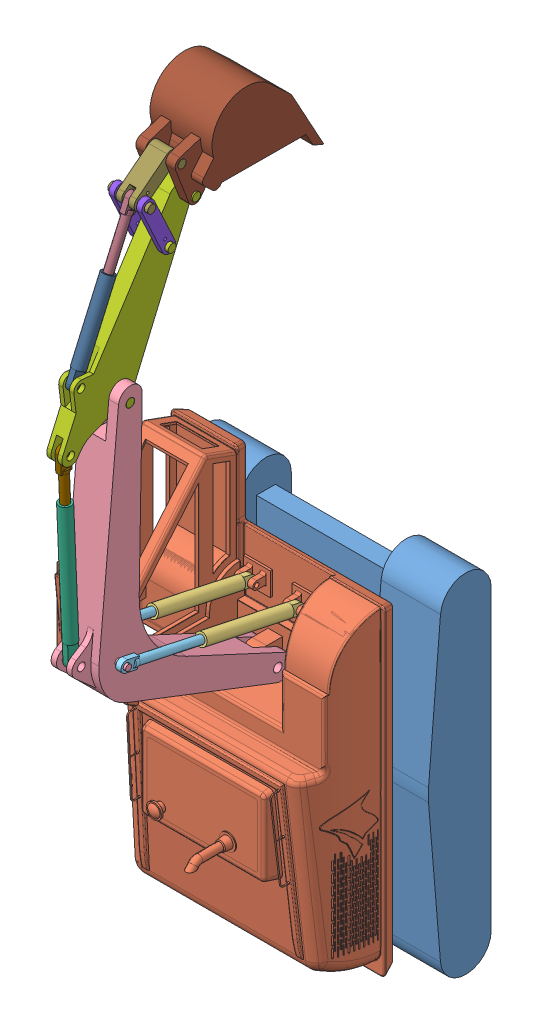
SolidWorks assembly MathScavator9000_nested, configuration Default. Lengths in mm.
Overall size (4800 14739.5 7058.03).
24 component instances, 13 part files, 2 mates.
Components (placement in the parent):
- ExcavatorBase-1: ExcavatorBase [Default] at origin size (4800 6440 1295)
- Chassis_Boom_Stick_Bucket_Assembly^MathScavator9000_nested-1: Chassis_Boom_Stick_Bucket_Assembly^MathScavator9000_nested [Default] at (-67.6256 -13.1371 -77.4342) size (3985.01 14479.39 5863.03) (virtual, flexible)
  - Chassis_BoomCyl^Chassis_Boom_Stick_Bucket_Assembly_MathScavator9000_nested-1: Chassis_BoomCyl^Chassis_Boom_Stick_Bucket_Assembly_MathScavator9000_nested [Default] at (67.6256 13.1371 77.4342) size (3985.01 7287.04 2544.86) (virtual, flexible)
    - Chassis_Primary_v2_PART-1: Chassis_Primary_v2_PART [Default] at origin size (3985.01 7287.04 2544.86)
    - BoomCyl-1: BoomCyl [Default] at (-446.0473 882.5913 372.5917) x (1 0 0) z (0 0.208273 0.978071) size (223.61 223.61 1900)
    - BoomCyl-2: BoomCyl [Default] at (453.9527 882.5913 372.5917) x (1 0 0) z (0 0.208273 0.978071) size (223.61 223.61 1900)
  - Boom_Stick_Bucket_assembly^Chassis_Boom_Stick_Bucket_Assembly_MathScavator9000_nested-1: Boom_Stick_Bucket_assembly^Chassis_Boom_Stick_Bucket_Assembly_MathScavator9000_nested [Default] at origin size (1148 11504.17 5802.13) (virtual, flexible)
    - Boom_BoomPiston_StickCyl^Boom_Stick_Bucket_assembly_Chassis_Boom_Stick_Bucket_Assembly_MathScavator9000_nested-1: Boom_BoomPiston_StickCyl^Boom_Stick_Bucket_assembly_Chassis_Boom_Stick_Bucket_Assembly_MathScavator9000_nested [Default] at origin size (1080 7332.45 5513.89) (virtual, flexible)
      - Boom-1: Boom [Default] at (71.5783 -4.2715 675.0259) x (0 0.899116 0.437711) z (1 0 0) size (6775.47 2834.12 1080)
      - BoomPiston-1: BoomPiston [Default] at (521.5783 1574.5137 3637.6672) x (1 0 0) z (0 0.208273 0.978071) size (163.61 200 2150)
      - BoomPiston-2: BoomPiston [Default] at (-378.4217 1574.5137 3637.6672) x (1 0 0) z (0 0.208273 0.978071) size (163.61 200 2150)
      - StickCyl-1: StickCyl [Default] at (73.5783 1678.5342 4163.5449) x (1 0 0) z (0 0.999081 0.042851) size (223.61 223.61 2700)
    - Stick_Bucket_assembly^Boom_Stick_Bucket_assembly_Chassis_Boom_Stick_Bucket_Assembly_MathScavator9000_nested-1: Stick_Bucket_assembly^Boom_Stick_Bucket_assembly_Chassis_Boom_Stick_Bucket_Assembly_MathScavator9000_nested [Default] at origin size (1148 7430.27 4651.1) (virtual, flexible)
      - Stick_StickLink_StickPiston_BucketCyl^Stick_Bucket_assembly_Boom_Stick_Bucket_assembly_Chassis_Boom_Stick_Bucket_Assembly_MathScavator9000_nested-1: Stick_StickLink_StickPiston_BucketCyl^Stick_Bucket_assembly_Boom_Stick_Bucket_assembly_Chassis_Boom_Stick_Bucket_Assembly_MathScavator9000_nested [Default] at origin size (780 6150.25 2715.92) (virtual, flexible)
        - Stick-1: Stick [Default] at (71.5783 5606.2108 3406.3421) x (0 0.920038 -0.39183) z (1 0 0) size (4089.97 1210.11 780)
        - StickLink-1: StickLink [Default] at (327.5783 7721.9511 2657.4476) x (1 0.00021 0.000097) z (0 -0.421504 0.906826) size (100.26 1142.82 240)
        - StickLink-2: StickLink [Default] at (-184.4217 7721.9511 2657.4476) x (1 0.00021 0.000097) z (0 -0.421504 0.906826) size (100.26 1142.82 240)
        - StickPiston-1: StickPiston [Default] at (73.5783 5104.4531 4310.4849) x (1 0 0) z (0 0.999081 0.042851) size (163.61 200 2500)
        - BucketCyl-1: BucketCyl [Default] at (71.5783 6090.2719 4117.0896) x (1 0 0) z (0 0.915184 -0.403037) size (223.61 223.61 1700)
      - Bucket_BucketLink_BucketPiston^Stick_Bucket_assembly_Boom_Stick_Bucket_assembly_Chassis_Boom_Stick_Bucket_Assembly_MathScavator9000_nested-1: Bucket_BucketLink_BucketPiston^Stick_Bucket_assembly_Boom_Stick_Bucket_assembly_Chassis_Boom_Stick_Bucket_Assembly_MathScavator9000_nested [Default] at origin size (1148 2990.58 2942.63) (virtual, flexible)
        - Bucket-1: Bucket [Default] at (66.3783 8343.955 2230.4406) x (0 0.868518 0.495658) z (1 0 0) size (2219.62 1959.94 1148)
        - BucketPiston_BucketLink^Bucket_BucketLink_BucketPiston_Stick_Bucket_assembly_Boom_Stick_Bucket_assembly_Chassis_Boom_Stick_Bucket_Assembly_MathScavator9000_nested-1: BucketPiston_BucketLink^Bucket_BucketLink_BucketPiston_Stick_Bucket_assembly_Boom_Stick_Bucket_assembly_Chassis_Boom_Stick_Bucket_Assembly_MathScavator9000_nested [Default] at (-56.421 -139.1745 -91.1582) size (738.42 1830.29 1699.85) (virtual, flexible)
          - BucketLink-1: BucketLink [Default] at (125.9513 8679.8042 3129.1377) x (1 -0.000008 0.00001) z (-0.000013 -0.617711 0.786405) size (738.41 251.24 966.87)
          - BucketPiston-1: BucketPiston [Default] at (127.9993 8679.8042 3129.1377) x (1 0 0) z (0 0.915184 -0.403037) size (163.61 200 1600)
Mates (geometry in assembly coordinates):
- Concentric34: concentric anti-aligned: cylinder of ExcavatorBase-1 through (0 0 0) axis (0 0 -1) radius 750; cylinder of Assem8^MathScavator9000_nested-1/Assem9^Assem8_MathScavator9000_nested-1/Chassis_Primary_v2_PART-1 through (0 0 -100) axis (0 0 1) radius 1250
- Coincident14: coincident anti-aligned: plane of ExcavatorBase-1 through (750 0 0) normal (0 0 1); plane of Assem8^MathScavator9000_nested-1/Assem9^Assem8_MathScavator9000_nested-1/Chassis_Primary_v2_PART-1 through (2005 863.5 0) normal (0 0 -1)
